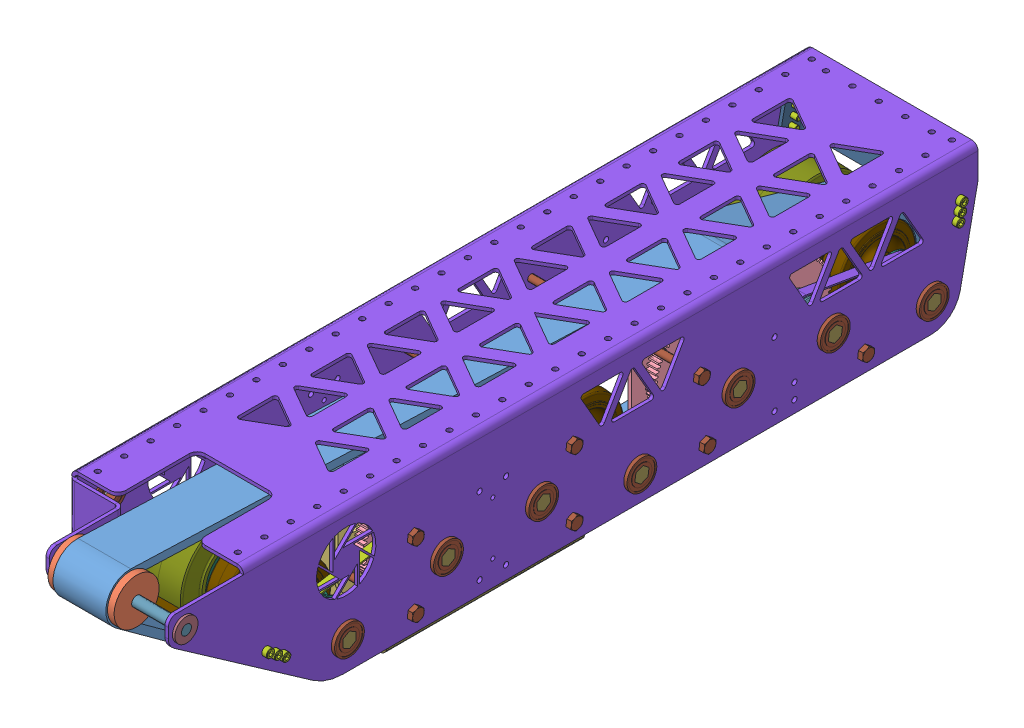
SolidWorks assembly 0001- 01 - 1001 DRIVE TRAIN FRAME NO MATES, configuration Default. Lengths in mm.
Overall size (218.31 373.88 795.79).
122 component instances, 31 part files, 19 mates.
Components (placement in the parent):
- 0001- 01 - 0001 Reference Geometry-1: 0001- 01 - 0001 Reference Geometry [Default] at origin size (111.12 355.6 787.4) (hidden)
- 0001- 01 - 1020 DRIVE ASSEMBLY-1: 0001- 01 - 1020 DRIVE ASSEMBLY [Default] at (102.3557 0 0) size (201.34 355.6 787.4)
  - 0001- 01 - 0001 Reference Geometry-1: 0001- 01 - 0001 Reference Geometry [Default] at origin size (111.12 355.6 787.4) (hidden)
  - MiniCIM-1: MiniCIM [Default] at (0 75.0243 -315.6349) x (-1 0 0) z (0 0.602963 -0.797769) size (125.82 64.01 64.01)
  - MiniCIM-2: MiniCIM [Default] at (0 75.0243 -595.7725) x (-1 0 0) z (0 -0.916851 0.39923) size (125.82 64.01 64.01)
  - Gear - 11t CIM-1: Gear - 11t CIM [Default] at (13.525 75.0243 -315.6349) x (0 -0.797769 -0.602963) z (1 0 0) size (17.96 18.15 19.05)
  - Gear - 11t CIM-2: Gear - 11t CIM [Default] at (13.525 75.0243 -595.7725) x (0 0.39923 0.916851) z (1 0 0) size (17.96 18.15 19.05)
  - MiniCIM Washer-1: MiniCIM Washer [Default] at (23.05 75.0243 -315.6349) x (1 0 0) z (0 0.588949 -0.808171) size (1.2 14.83 14.83)
  - MiniCIM Washer-2: MiniCIM Washer [Default] at (23.05 75.0243 -595.7725) x (1 0 0) z (0 0.909743 -0.415171) size (1.2 14.83 14.83)
  - Gear - 60t-1: Gear - 60t [Default] at (18.2875 75.0243 -269.9149) x (0 -0.768183 -0.640231) z (-1 0 0) size (78.95 78.95 12.65)
  - Gear - 60t-2: Gear - 60t [Default] at (18.2875 75.0243 -361.3549) x (0 0.487746 0.872986) z (-1 0 0) size (78.95 78.95 12.65)
  - Gear - 60t-3: Gear - 60t [Default] at (18.2875 75.0243 -550.0525) x (0 0.991481 0.130252) z (-1 0 0) size (78.95 78.95 12.65)
  - Gear - 60t-4: Gear - 60t [Default] at (18.2875 75.0243 -641.4925) x (0 0.177919 -0.984045) z (-1 0 0) size (78.95 78.95 12.65)
  - Pulley - 18t-1: Pulley - 18t [Default] at (31.8621 75.0243 -269.9149) x (0 0.34515 0.938547) z (-1 0 0) size (32 32 14.5)
  - Pulley - 18t-2: Pulley - 18t [Default] at (31.8621 75.0243 -361.3549) x (0 0.872986 -0.487746) z (1 0 0) size (32 32 14.5)
  - Pulley - 18t-3: Pulley - 18t [Default] at (46.3401 75.0243 -550.0525) x (0 -0.923774 0.382939) z (1 0 0) size (32 32 14.5)
  - Pulley - 18t-4: Pulley - 18t [Default] at (31.8621 75.0243 -641.4925) x (0 -0.33794 -0.941168) z (-1 0 0) size (32 32 14.5)
  - Pulley - 24t-1: Pulley - 24t [Default] at (31.8621 53.975 -174.8073) x (0 -0.163539 0.986537) z (-1 0 0) size (42 42 14.5)
  - Pulley - 24t-2: Pulley - 24t [Default] at (31.8621 50.8 -455.7037) x (0 -0.971432 -0.237319) z (-1 0 0) size (42 42 14.5)
  - Pulley - 24t-3: Pulley - 24t [Default] at (31.8621 53.975 -736.6) x (0 0.533781 -0.845622) z (-1 0 0) size (42 42 14.5)
  - Pulley - 24t-4: Pulley - 24t [Default] at (46.3621 50.8 -455.7037) x (0 -0.971432 -0.237319) z (-1 0 0) size (42 42 14.5)
  - Belt1-11^0001- 01 - 1020 DRIVE ASSEMBLY-1: Belt1-11^0001- 01 - 1020 DRIVE ASSEMBLY [Default] at (26.3621 38.4825 -184.9631) x (0 0 -1) z (1 0 0) size (132.28 58.22 9) (virtual)
  - Belt4-14^0001- 01 - 1020 DRIVE ASSEMBLY-1: Belt4-14^0001- 01 - 1020 DRIVE ASSEMBLY [Default] at (26.3621 70.7168 -630.5861) x (0 0 -1) z (1 0 0) size (132.28 58.22 9) (virtual)
  - Belt2-12-2: Belt2-12 [Default] at (26.1746 76.9004 -347.844) x (0 0 -1) z (1 0 0) size (131.52 61.39 9)
  - Belt3-13-2: Belt3-13 [Default] at (41.6721 37.9854 -445.3032) x (0 0 -1) z (1 0 0) size (131.52 61.39 9)
- 0001- 01 - 1030 BEARINGS AND AXLES-1: 0001- 01 - 1030 BEARINGS AND AXLES [Default] at origin size (171.45 355.6 787.4)
  - 0001- 01 - 0001 Reference Geometry-1: 0001- 01 - 0001 Reference Geometry [Default] at origin size (111.12 355.6 787.4) (hidden)
  - Bearing - 0.5 Hex Flanged-1: Bearing - 0.5 Hex Flanged [Default] at (-3.175 75.0243 -641.4925) x (0 0.990292 -0.139005) z (0 -0.139005 -0.990292) size (31.12 7.94 31.12)
  - Bearing - 0.5 Hex Flanged-2: Bearing - 0.5 Hex Flanged [Default] at (-3.175 53.975 -174.8073) x (0 -1 0) z (0 0 1) size (31.12 7.94 31.12)
  - Bearing - 0.5 Hex Flanged-3: Bearing - 0.5 Hex Flanged [Default] at (-3.175 50.8 -455.7037) x (0 -0.617689 -0.786423) z (0 -0.786423 0.617689) size (31.12 7.94 31.12)
  - Bearing - 0.5 Hex Flanged-4: Bearing - 0.5 Hex Flanged [Default] at (-3.175 75.0243 -550.0525) x (0 -0.995157 -0.098298) z (0 -0.098298 0.995157) size (31.12 7.94 31.12)
  - Bearing - 0.5 Hex Flanged-5: Bearing - 0.5 Hex Flanged [Default] at (-3.175 53.975 -736.6) x (0 -1 0) z (0 0 1) size (31.12 7.94 31.12)
  - Bearing - 0.5 Hex Flanged-6: Bearing - 0.5 Hex Flanged [Default] at (-3.175 75.0243 -269.9149) x (0 -1 0) z (0 0 1) size (31.12 7.94 31.12)
  - Bearing - 0.5 Hex Flanged-7: Bearing - 0.5 Hex Flanged [Default] at (-3.175 75.0243 -361.3549) x (0 -0.995055 -0.099325) z (0 -0.099325 0.995055) size (31.12 7.94 31.12)
  - 0001- 01 - 1031 Hex Axle 6.75x0.5-1: 0001- 01 - 1031 Hex Axle 6.75x0.5 [Default] at (168.275 53.9703 -174.8046) x (-1 0 0) z (0 0.5 0.866025) size (171.45 12.73 14.69)
  - 0001- 01 - 1031 Hex Axle 6.75x0.5-2: 0001- 01 - 1031 Hex Axle 6.75x0.5 [Default] at (-3.175 75.029 -269.9176) x (1 0 0) z (0 -0.5 0.866025) size (171.45 12.73 14.69)
  - 0001- 01 - 1031 Hex Axle 6.75x0.5-3: 0001- 01 - 1031 Hex Axle 6.75x0.5 [Default] at (-3.175 75.0287 -361.3517) x (1 0 0) z (0 0.41151 0.911405) size (171.45 12.73 14.69)
  - 0001- 01 - 1031 Hex Axle 6.75x0.5-4: 0001- 01 - 1031 Hex Axle 6.75x0.5 [Default] at (-3.175 50.8008 -455.6983) x (1 0 0) z (0 0.372218 -0.928146) size (171.45 12.73 14.69)
  - 0001- 01 - 1031 Hex Axle 6.75x0.5-5: 0001- 01 - 1031 Hex Axle 6.75x0.5 [Default] at (-3.175 75.0225 -550.0499) x (1 0 0) z (0 -0.582707 0.812682) size (171.45 12.73 14.69)
  - 0001- 01 - 1031 Hex Axle 6.75x0.5-6: 0001- 01 - 1031 Hex Axle 6.75x0.5 [Default] at (-3.175 53.9703 -736.5973) x (1 0 0) z (0 0.5 -0.866025) size (171.45 12.73 14.69)
  - 0001- 01 - 1031 Hex Axle 6.75x0.5-7: 0001- 01 - 1031 Hex Axle 6.75x0.5 [Default] at (-3.175 75.025 -641.4871) x (1 0 0) z (0 0.990292 -0.139005) size (171.45 12.73 14.69)
  - Bearing - 0.5 Hex Flanged-8: Bearing - 0.5 Hex Flanged [Default] at (168.275 53.975 -174.8073) x (0 1 0) z (0 0 1) size (31.12 7.94 31.12)
  - Bearing - 0.5 Hex Flanged-9: Bearing - 0.5 Hex Flanged [Default] at (168.275 75.0243 -269.9203) x (0 1 0) z (0 0 1) size (31.12 7.94 31.12)
  - Bearing - 0.5 Hex Flanged-10: Bearing - 0.5 Hex Flanged [Default] at (168.275 50.805 -455.7017) x (0 -0.989906 0.141723) z (0 -0.141723 -0.989906) size (31.12 7.94 31.12)
  - Bearing - 0.5 Hex Flanged-11: Bearing - 0.5 Hex Flanged [Default] at (168.275 75.0238 -361.3495) x (0 -0.995055 -0.099325) z (0 0.099325 -0.995055) size (31.12 7.94 31.12)
  - Bearing - 0.5 Hex Flanged-12: Bearing - 0.5 Hex Flanged [Default] at (168.275 75.0181 -550.0531) x (0 0.995157 0.098298) z (0 -0.098298 0.995157) size (31.12 7.94 31.12)
  - Bearing - 0.5 Hex Flanged-13: Bearing - 0.5 Hex Flanged [Default] at (168.275 75.0208 -641.4838) x (0 0.990292 -0.139005) z (0 0.139005 0.990292) size (31.12 7.94 31.12)
  - Bearing - 0.5 Hex Flanged-14: Bearing - 0.5 Hex Flanged [Default] at (168.275 53.975 -736.6) x (0 1 0) z (0 0 1) size (31.12 7.94 31.12)
  - Bearing - 0.875 Flanged-1: Bearing - 0.875 Flanged [Default] at (46.0375 139.7817 -19.05) size (7.11 24.61 24.61)
  - Bearing - 0.875 Flanged-2: Bearing - 0.875 Flanged [Default] at (160.3375 139.7817 -19.05) size (7.11 24.61 24.61)
  - 0001- 01 - 1032 Axle 4.75x0.375-1: 0001- 01 - 1032 Axle 4.75x0.375 [Default] at (46.7995 139.7817 -19.05) x (1 0 0) z (0 0.031061 0.999517) size (120.65 9.53 9.53)
  - Bearing - 0.5 Hex Flanged-15: Bearing - 0.5 Hex Flanged [Default] at (-3.175 126.365 -109.6291) x (0 -1 0) z (0 0 1) size (31.12 7.94 31.12)
- 0001- 01 - 1040 WHEEL ASSEMBLY-1: 0001- 01 - 1040 WHEEL ASSEMBLY [Default] at (4.4625 0 0) size (115.1 373.88 795.79)
  - 0001- 01 - 0001 Reference Geometry-1: 0001- 01 - 0001 Reference Geometry [Default] at origin size (111.12 355.6 787.4) (hidden)
  - Colson - 4 x 2 Hex-1: Colson - 4 x 2 Hex [Default] at (28.9766 50.8 -455.7037) x (1 0 0) z (0 -0.557084 0.830456) size (57.95 99.57 99.57)
    - Colson - 4 x 2 Hex 03-1: Colson - 4 x 2 Hex 03 [Default] at origin size (55.55 82.55 82.55)
    - Colson - 4 x 2 Hex 01-1: Colson - 4 x 2 Hex 01 [Default] at origin size (50.8 99.57 99.57)
    - Colson - 4 x 2 Hex 02-1: Colson - 4 x 2 Hex 02 [Default] x (0 0 1) z (-1 0 0) size (50.79 50.79 57.95)
  - Colson - 4 x 2 Hex-2: Colson - 4 x 2 Hex [Default] at (28.9766 53.975 -736.6) x (1 0 0) z (0 -0.049345 -0.998782) size (57.95 99.57 99.57)
    - Colson - 4 x 2 Hex 03-1: Colson - 4 x 2 Hex 03 [Default] at origin size (55.55 82.55 82.55)
    - Colson - 4 x 2 Hex 01-1: Colson - 4 x 2 Hex 01 [Default] at origin size (50.8 99.57 99.57)
    - Colson - 4 x 2 Hex 02-1: Colson - 4 x 2 Hex 02 [Default] x (0 0 1) z (-1 0 0) size (50.79 50.79 57.95)
  - Colson - 4 x 2 Hex-3: Colson - 4 x 2 Hex [Default] at (28.9766 53.975 -174.8073) x (1 0 0) z (0 0.745926 -0.666029) size (57.95 99.57 99.57)
    - Colson - 4 x 2 Hex 03-1: Colson - 4 x 2 Hex 03 [Default] at origin size (55.55 82.55 82.55)
    - Colson - 4 x 2 Hex 01-1: Colson - 4 x 2 Hex 01 [Default] at origin size (50.8 99.57 99.57)
    - Colson - 4 x 2 Hex 02-1: Colson - 4 x 2 Hex 02 [Default] x (0 0 1) z (-1 0 0) size (50.79 50.79 57.95)
  - Colson - 3 x 0.875 Hex-1: Colson - 3 x 0.875 Hex [Default] at (71.7469 53.975 -174.8073) x (0 0.203834 0.979005) z (-1 0 0) size (76.2 76.2 27.59)
  - Colson - 3 x 0.875 Hex-2: Colson - 3 x 0.875 Hex [Default] at (99.3345 53.975 -174.8073) x (0 0.203834 0.979005) z (-1 0 0) size (76.2 76.2 27.59)
  - Colson - 3 x 0.875 Hex-3: Colson - 3 x 0.875 Hex [Default] at (71.7469 50.8 -455.7037) x (0 -0.557084 0.830456) z (-1 0 0) size (76.2 76.2 27.59)
  - Colson - 3 x 0.875 Hex-4: Colson - 3 x 0.875 Hex [Default] at (99.3345 50.8 -455.7037) x (0 -0.557084 0.830456) z (-1 0 0) size (76.2 76.2 27.59)
  - Colson - 3 x 0.875 Hex-5: Colson - 3 x 0.875 Hex [Default] at (99.3345 53.975 -736.6) x (0 -0.049345 -0.998782) z (-1 0 0) size (76.2 76.2 27.59)
  - Colson - 3 x 0.875 Hex-6: Colson - 3 x 0.875 Hex [Default] at (71.7469 53.975 -736.6) x (0 -0.049345 -0.998782) z (-1 0 0) size (76.2 76.2 27.59)
  - 0001- 01 - 1041 Tread-1: 0001- 01 - 1041 Tread [Default] at (57.9532 0 0) size (50.8 157.69 786.26)
  - 0001- 01 - 1042 Top Pulley-1: 0001- 01 - 1042 Top Pulley [Default] at (51.6032 139.7817 -19.05) x (1 0 0) z (0 0.971922 -0.235302) size (63.5 43.18 43.18)
- 0001- 01 - 1050 MOUNTING ASSEMBLY-1: 0001- 01 - 1050 MOUNTING ASSEMBLY [Default] at (102.3557 0 0) size (171.45 355.6 787.4)
  - 0001- 01 - 0001 Reference Geometry-1: 0001- 01 - 0001 Reference Geometry [Default] at origin size (111.12 355.6 787.4) (hidden)
  - 0001- 01 - 1051 CIM Mounting Plate-1: 0001- 01 - 1051 CIM Mounting Plate [Default] at origin size (3.17 88.9 177.8)
  - 0001- 01 - 1052 CIM Mounting Plate Back-1: 0001- 01 - 1052 CIM Mounting Plate Back [Default] at origin size (3.18 85.92 177.8)
  - 0001- 01 - 1053 CIM Mounting Plate Outer-1: 0001- 01 - 1053 CIM Mounting Plate Outer [Default] at (-55.5625 0 0) size (3.18 88.9 177.8)
  - 0001- 01 - 1054 CIM Mounting Plate Outer Back-1: 0001- 01 - 1054 CIM Mounting Plate Outer Back [Default] at (-55.5625 0 0) size (3.18 80.08 177.8)
  - socket head cap screw_ai-2: socket head cap screw_ai [HX-SHCS 0.19-32x2.5x1.125-N] at (9.5885 36.9243 -586.2475) x (-1 0 0) z (0 0.924225 0.381849) size (68.33 7.94 7.94)
  - socket head cap screw_ai-3: socket head cap screw_ai [HX-SHCS 0.19-32x2.5x1.125-N] at (9.5885 36.9243 -605.2975) x (-1 0 0) z (0 0.924225 0.381849) size (68.33 7.94 7.94)
  - socket head cap screw_ai-4: socket head cap screw_ai [HX-SHCS 0.19-32x2.5x1.125-N] at (8.001 38.1943 -302.9349) x (-1 0 0) z (0 0.924225 0.381849) size (68.33 7.94 7.94)
  - socket head cap screw_ai-5: socket head cap screw_ai [HX-SHCS 0.19-32x2.5x1.125-N] at (8.001 38.1943 -328.3349) x (-1 0 0) z (0 0.924225 0.381849) size (68.33 7.94 7.94)
  - socket head cap screw_ai-6: socket head cap screw_ai [HX-SHCS 0.19-32x2.5x1.125-N] at (8.001 111.8543 -328.3349) x (-1 0 0) z (0 0.924225 0.381849) size (68.33 7.94 7.94)
  - socket head cap screw_ai-7: socket head cap screw_ai [HX-SHCS 0.19-32x2.5x1.125-N] at (8.001 111.8543 -302.9349) x (-1 0 0) z (0 0.924225 0.381849) size (68.33 7.94 7.94)
  - socket head cap screw_ai-8: socket head cap screw_ai [HX-SHCS 0.19-32x0.5x0.5-N] at (9.5885 98.5707 -586.2475) x (-1 0 0) z (0 0.924225 0.381849) size (17.53 7.94 7.94)
  - socket head cap screw_ai-9: socket head cap screw_ai [HX-SHCS 0.19-32x0.5x0.5-N] at (9.5885 51.4779 -605.2975) x (-1 0 0) z (0 0.924225 0.381849) size (17.53 7.94 7.94)
  - socket head cap screw_ai-10: socket head cap screw_ai [HX-SHCS 0.19-32x0.5x0.5-N] at (8.001 49.6243 -315.6349) x (-1 0 0) z (0 0.924225 0.381849) size (17.53 7.94 7.94)
  - socket head cap screw_ai-11: socket head cap screw_ai [HX-SHCS 0.19-32x0.5x0.5-N] at (8.001 100.4243 -315.6349) x (-1 0 0) z (0 0.924225 0.381849) size (17.53 7.94 7.94)
- 0001- 01 - 1060 FRAME ASSEMBLY-1: 0001- 01 - 1060 FRAME ASSEMBLY [Default] at origin size (174.75 355.6 787.4)
  - 0001- 01 - 0001 Reference Geometry-1: 0001- 01 - 0001 Reference Geometry [Default] at origin size (111.12 355.6 787.4) (hidden)
  - 0001- 01 - 1010 Drive Frame-1: 0001- 01 - 1010 Drive Frame [Default] at origin size (165.1 136.61 777.68)
  - 0001- 01 - 1011 Frame Support Front-1: 0001- 01 - 1011 Frame Support Front [Default] at (3.175 0 0) size (158.75 37.46 42.14)
  - 0001- 01 - 1012 Frame Support Back-1: 0001- 01 - 1012 Frame Support Back [Default] at (3.175 0 0) size (158.75 36.23 31.29)
  - socket head cap screw_ai-1: socket head cap screw_ai [HX-SHCS 0.19-32x0.5x0.5-N] at (169.926 123.8969 -763.9866) x (-1 0 0) z (0 0.924225 0.381849) size (17.53 7.94 7.94)
  - socket head cap screw_ai-2: socket head cap screw_ai [HX-SHCS 0.19-32x0.5x0.5-N] at (169.926 116.123 -762.3835) x (-1 0 0) z (0 0.924225 0.381849) size (17.53 7.94 7.94)
  - socket head cap screw_ai-3: socket head cap screw_ai [HX-SHCS 0.19-32x0.5x0.5-N] at (169.926 108.3491 -760.7803) x (-1 0 0) z (0 0.924225 0.381849) size (17.53 7.94 7.94)
  - socket head cap screw_ai-4: socket head cap screw_ai [HX-SHCS 0.19-32x0.5x0.5-N] at (-4.826 123.8969 -763.9866) size (17.53 7.94 7.94)
  - socket head cap screw_ai-5: socket head cap screw_ai [HX-SHCS 0.19-32x0.5x0.5-N] at (-4.826 116.123 -762.3835) size (17.53 7.94 7.94)
  - socket head cap screw_ai-6: socket head cap screw_ai [HX-SHCS 0.19-32x0.5x0.5-N] at (-4.826 108.3491 -760.7803) size (17.53 7.94 7.94)
  - socket head cap screw_ai-7: socket head cap screw_ai [HX-SHCS 0.19-32x0.5x0.5-N] at (-4.826 81.7927 -97.7153) x (1 0 0) z (0 -0.557697 0.830044) size (17.53 7.94 7.94)
  - socket head cap screw_ai-8: socket head cap screw_ai [HX-SHCS 0.19-32x0.5x0.5-N] at (-4.826 76.3294 -105.5177) size (17.53 7.94 7.94)
  - socket head cap screw_ai-9: socket head cap screw_ai [HX-SHCS 0.19-32x0.5x0.5-N] at (-4.826 70.8661 -113.3202) size (17.53 7.94 7.94)
  - socket head cap screw_ai-11: socket head cap screw_ai [HX-SHCS 0.19-32x0.5x0.5-N] at (169.926 81.7927 -97.7153) x (-1 0 0) z (0 0.924225 0.381849) size (17.53 7.94 7.94)
  - socket head cap screw_ai-12: socket head cap screw_ai [HX-SHCS 0.19-32x0.5x0.5-N] at (169.926 76.3294 -105.5177) x (-1 0 0) z (0 0.924225 0.381849) size (17.53 7.94 7.94)
  - socket head cap screw_ai-13: socket head cap screw_ai [HX-SHCS 0.19-32x0.5x0.5-N] at (169.926 70.8661 -113.3202) x (-1 0 0) z (0 0.924225 0.381849) size (17.53 7.94 7.94)
  - hex bolt_ai-1: hex bolt_ai [HBOLT 0.2500-20x2.5x0.75-N] at (169.8752 106.7743 -239.4349) x (-1 0 0) z (0 0.924225 0.381849) size (68.28 12.85 11.13)
  - hex bolt_ai-3: hex bolt_ai [HBOLT 0.2500-20x2.5x0.75-N] at (169.8752 106.7743 -391.8349) x (-1 0 0) z (0 0.924225 0.381849) size (68.28 12.85 11.13)
  - hex bolt_ai-4: hex bolt_ai [HBOLT 0.2500-20x2.5x0.75-N] at (169.8752 43.2743 -391.8349) x (-1 0 0) z (0 0.924225 0.381849) size (68.28 12.85 11.13)
  - hex bolt_ai-5: hex bolt_ai [HBOLT 0.2500-20x2.5x0.75-N] at (169.8752 43.2743 -239.4349) x (-1 0 0) z (0 0.924225 0.381849) size (68.28 12.85 11.13)
  - hex bolt_ai-6: hex bolt_ai [HBOLT 0.2500-20x2.5x0.75-N] at (169.8752 102.9745 -514.2182) x (-1 0 0) z (0 0.924225 0.381849) size (68.28 12.85 11.13)
  - hex bolt_ai-7: hex bolt_ai [HBOLT 0.2500-20x2.5x0.75-N] at (169.8752 43.2743 -519.5725) x (-1 0 0) z (0 0.924225 0.381849) size (68.28 12.85 11.13)
  - hex bolt_ai-8: hex bolt_ai [HBOLT 0.2500-20x2.5x0.75-N] at (169.8752 43.2743 -671.9725) x (-1 0 0) z (0 0.924225 0.381849) size (68.28 12.85 11.13)
  - hex bolt_ai-9: hex bolt_ai [HBOLT 0.2500-20x2x2-N] at (-4.7752 106.7743 -239.4349) size (55.58 12.85 11.13)
  - hex bolt_ai-10: hex bolt_ai [HBOLT 0.2500-20x2x2-N] at (-4.7752 43.2743 -239.4349) size (55.58 12.85 11.13)
  - hex bolt_ai-11: hex bolt_ai [HBOLT 0.2500-20x2x2-N] at (-4.7752 43.2743 -391.8349) size (55.58 12.85 11.13)
  - hex bolt_ai-12: hex bolt_ai [HBOLT 0.2500-20x2x2-N] at (-4.7752 106.7743 -391.8349) size (55.58 12.85 11.13)
  - hex bolt_ai-13: hex bolt_ai [HBOLT 0.2500-20x2x2-N] at (-4.7752 102.9745 -514.2182) size (55.58 12.85 11.13)
  - hex bolt_ai-14: hex bolt_ai [HBOLT 0.2500-20x2x2-N] at (-4.7752 43.2743 -519.5725) size (55.58 12.85 11.13)
  - hex bolt_ai-15: hex bolt_ai [HBOLT 0.2500-20x2x2-N] at (-4.7752 43.2743 -671.9725) size (55.58 12.85 11.13)
- 0001- 01 - 1057 Bottom Tensioner-1: 0001- 01 - 1057 Bottom Tensioner [Default] at (82.55 31.8292 -407.2016) size (158.75 30.48 190.5)
Mates (geometry in assembly coordinates):
- Coincident1: coincident aligned: plane of 0001- 01 - 0001 Reference Geometry-1 through (0 0 0) normal (0 0 1); plane of assembly through (0 0 0) normal (0 0 1)
- Coincident2: coincident aligned: plane of 0001- 01 - 0001 Reference Geometry-1 through (0 0 0) normal (0 1 0); plane of assembly through (0 0 0) normal (0 1 0)
- Coincident3: coincident aligned: plane of 0001- 01 - 0001 Reference Geometry-1 through (0 0 0) normal (1 0 0); plane of assembly through (0 0 0) normal (1 0 0)
- Coincident4: coincident aligned: plane of 0001- 01 - 1020 DRIVE ASSEMBLY-1/0001- 01 - 0001 Reference Geometry-1 through (102.3557 0 0) normal (0 0 1); plane of assembly through (0 0 0) normal (0 0 1)
- Coincident5: coincident aligned: plane of 0001- 01 - 1020 DRIVE ASSEMBLY-1/0001- 01 - 0001 Reference Geometry-1 through (102.3557 0 0) normal (0 1 0); plane of assembly through (0 0 0) normal (0 1 0)
- Coincident7: coincident aligned: plane of 0001- 01 - 1030 BEARINGS AND AXLES-1/0001- 01 - 0001 Reference Geometry-1 through (0 0 0) normal (0 0 1); plane of assembly through (0 0 0) normal (0 0 1)
- Coincident8: coincident aligned: plane of 0001- 01 - 1030 BEARINGS AND AXLES-1/0001- 01 - 0001 Reference Geometry-1 through (0 0 0) normal (0 1 0); plane of assembly through (0 0 0) normal (0 1 0)
- Coincident9: coincident aligned: plane of 0001- 01 - 1030 BEARINGS AND AXLES-1/0001- 01 - 0001 Reference Geometry-1 through (0 0 0) normal (1 0 0); plane of assembly through (0 0 0) normal (1 0 0)
- Coincident10: coincident aligned: plane of 0001- 01 - 1040 WHEEL ASSEMBLY-1/0001- 01 - 0001 Reference Geometry-1 through (4.4625 0 0) normal (0 0 1); plane of assembly through (0 0 0) normal (0 0 1)
- Coincident11: coincident aligned: plane of 0001- 01 - 1040 WHEEL ASSEMBLY-1/0001- 01 - 0001 Reference Geometry-1 through (4.4625 0 0) normal (0 1 0); plane of assembly through (0 0 0) normal (0 1 0)
- Coincident13: coincident anti-aligned: plane of 0001- 01 - 1030 BEARINGS AND AXLES-1/Bearing - 0.5 Hex Flanged-2 through (4.7625 41.275 -174.8073) normal (1 0 0); plane of 0001- 01 - 1040 WHEEL ASSEMBLY-1/Colson - 4 x 2 Hex-3/Colson - 4 x 2 Hex 02-1 through (4.7625 53.975 -174.8073) normal (-1 0 0)
- Coincident14: coincident aligned: plane of ? through (102.3557 0 0) normal (0 0 1); plane of assembly through (0 0 0) normal (0 0 1)
- Coincident15: coincident aligned: plane of ? through (102.3557 0 0) normal (0 1 0); plane of assembly through (0 0 0) normal (0 1 0)
- Coincident17: coincident anti-aligned: plane of 0001- 01 - 1020 DRIVE ASSEMBLY-1/MiniCIM-1 through (102.3557 82.623 -309.8916) normal (1 0 0); plane of ? through (102.3557 106.7743 -239.4349) normal (-1 0 0)
- Coincident18: coincident aligned: plane of ? through (0 0 0) normal (0 0 1); plane of assembly through (0 0 0) normal (0 0 1)
- Coincident19: coincident aligned: plane of ? through (0 0 0) normal (1 0 0); plane of assembly through (0 0 0) normal (1 0 0)
- Coincident20: coincident aligned: plane of ? through (0 0 0) normal (0 1 0); plane of assembly through (0 0 0) normal (0 1 0)
- Coincident22: coincident anti-aligned: plane of ? through (102.3557 106.7743 -239.4349) normal (-1 0 0); circle of 0001- 01 - 1060 FRAME ASSEMBLY-1/hex bolt_ai-1
- Coincident23: coincident anti-aligned: plane of ? through (161.925 0 0) normal (-1 0 0); plane of 0001- 01 - 1057 Bottom Tensioner-1 through (161.925 16.5892 -216.7016) normal (1 0 0)
